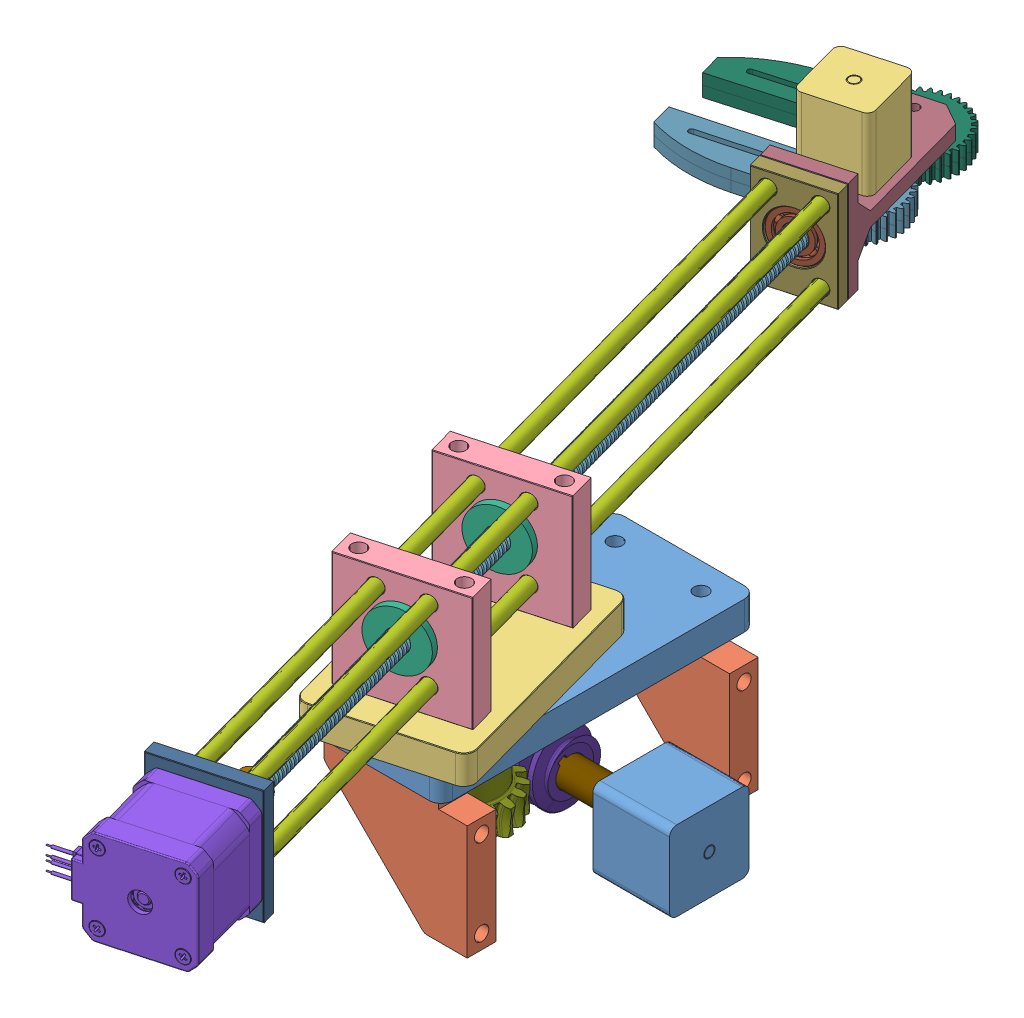
SolidWorks assembly CubeClawAssy, configuration Default. Lengths in mm.
Overall size (227.38 147.32 508.61).
29 component instances, 21 part files, 65 mates.
Components (placement in the parent):
- ClawArmBearingMount-1: ClawArmBearingMount [Default] at (-152.4 31.877 44.45) x (0 0 1) z (-1 0 0) size (139.7 12.7 63.5)
- 60355K509_BALL BEARING-1: 60355K509_BALL BEARING [60355K509] at (-152.4 36.6395 73.406) x (-0.297226 0 -0.954807) z (0 1 0) size (50.8 50.8 9.53)
- ArmRotate-1: ArmRotate [Default] at (-152.4 57.277 73.406) x (0.265648 0 0.96407) z (0.96407 0 -0.265648) size (101.6 63.5 63.5)
- RackStand-1: RackStand [Default] at (-160.8343 57.277 42.7968) x (0.265648 0 0.96407) z (-0.96407 0 0.265648) size (12 50.8 50.8)
- RackStand-2: RackStand [Default] at (-143.9657 57.277 104.0152) x (0.265648 0 0.96407) z (-0.96407 0 0.265648) size (12 50.8 50.8)
- 93410A912_ASTM A193 STEEL ACME LEAD SCREW-1: 93410A912_ASTM A193 STEEL ACME LEAD SCREW [93410A912] at (-159.5487 84.582 47.4626) x (0.957787 0.113984 -0.263917) z (-0.265648 0 -0.96407) size (11 9.53 384.84)
- 95120A592_BRONZE GENERAL PURPOSE ACME FLANGE NUT-1: 95120A592_BRONZE GENERAL PURPOSE ACME FLANGE NUT [95120A592] at (-158.3968 84.582 51.643) x (0.935858 -0.240148 -0.257875) z (0.231519 0.970736 -0.063795) size (25.4 22.84 25.4)
- 95120A592_BRONZE GENERAL PURPOSE ACME FLANGE NUT-2: 95120A592_BRONZE GENERAL PURPOSE ACME FLANGE NUT [95120A592] at (-141.5281 84.582 112.8615) x (0.890426 -0.383331 -0.245356) z (0.369558 0.923611 -0.101831) size (25.4 22.84 25.4)
- Rail-1: Rail [Default] at (-200.9719 68.707 -138.723) x (0.963827 0.022472 -0.265581) z (0.265648 0 0.96407) size (6.35 6.35 381)
- Rail-2: Rail [Default] at (-219.3375 68.707 -133.6624) x (0.963827 0.022472 -0.265581) z (0.265648 0 0.96407) size (6.35 6.35 381)
- Rail-3: Rail [Default] at (-219.3375 100.457 -133.6624) x (-0.624115 0.762171 0.171974) z (0.265648 0 0.96407) size (6.35 6.35 381)
- Rail-4: Rail [Default] at (-200.9719 100.457 -138.723) x (0.963827 0.022472 -0.265581) z (0.265648 0 0.96407) size (6.35 6.35 381)
- nema_17_motor-1: nema_17_motor [Varsayılan] at (-108.9426 84.582 231.1179) x (0 -1 0) z (-0.265648 0 -0.96407) size (42 58.5 65.65)
- ClawWormCoupler-1: ClawWormCoupler [Default] at (-117.5497 84.582 199.8821) x (0.587821 0.792611 -0.161973) z (0.265648 0 0.96407) size (13.97 13.97 25.4)
- ClawRailMotorBracket-1: ClawRailMotorBracket [Default] at (-110.6295 84.582 224.9961) x (0.96407 0 -0.265648) z (0.265648 0 0.96407) size (43.18 50.8 6.35)
- 60355K504_BALL BEARING-1: 60355K504_BALL BEARING [60355K504] at (-209.4167 84.582 -133.5144) x (-0.963827 -0.022472 0.265581) z (0.265648 0 0.96407) size (22.23 22.23 5.56)
- ClawBracket-1: ClawBracket [Default] at (-210.1547 84.582 -136.1927) x (0.96407 0 -0.265648) z (0.265648 0 0.96407) size (31.75 44.45 6.35)
- ClawMount-1: ClawMount [Default] at (-194.8501 62.357 -140.4099) x (-0.96407 0 0.265648) z (-0.265648 0 -0.96407) size (31.75 44.45 76.2)
- CLAW_L-1: CLAW_L [Default] at (-218.589 76.6445 -166.8019) x (-0.262286 0 -0.96499) z (0 -1 0) size (40.21 91.53 4.76)
- CLAW_L-2: CLAW_L [Default] at (-218.589 81.407 -166.8019) x (-0.262286 0 -0.96499) z (0 -1 0) size (40.21 91.53 4.76)
- CLAW_R-1: CLAW_R [Default] at (-228.7102 76.6445 -203.533) x (-0.274481 0 -0.961592) z (0 -1 0) size (40.15 91.5 4.76)
- CLAW_R-2: CLAW_R [Default] at (-228.7102 81.407 -203.533) x (-0.274481 0 -0.961592) z (0 -1 0) size (40.15 91.5 4.76)
- 57545K511_SPEED-REDUCING WORM GEAR FOR 90 DEG TRANSFER-1: 57545K511_SPEED-REDUCING WORM GEAR FOR 90 DEG TRANSFER [57545K511] at (-152.4 0.127 73.406) x (-0.122179 0 0.992508) z (-0.992508 0 -0.122179) size (44.78 28.61 44.18)
- 57545K527_SPEED-REDUCING WORM GEAR FOR 90 DEG TRANSFER-2: 57545K527_SPEED-REDUCING WORM GEAR FOR 90 DEG TRANSFER [57545K527] at (-151.281 0.382 40.4015) x (0 0.509771 -0.86031) z (1 0 0) size (31.13 29.72 30.93)
- RotationBushing-1: RotationBushing [Default] at (-111.5935 0.382 40.4015) x (0 -0.164114 0.986441) z (-1 0 0) size (12.7 12.7 53.98)
- 6627T380_POSITION-CONTROL DC MOTOR-1: 6627T380_POSITION-CONTROL DC MOTOR [6627T38] at (-109.5615 0.382 40.4015) x (0 0 1) z (-1 0 0) size (35.31 35.31 49.28)
- CubeArmMountBracket-3: CubeArmMountBracket [Default] at (-127 25.527 -7.3307) x (0 -1 0) z (0 0 -1) size (57.15 63.5 12.7)
- CubeArmMountBracket-4: CubeArmMountBracket [Default] at (-127 25.273 109.0013) x (0 -1 0) z (0 0 -1) size (57.15 63.5 12.7)
- 6627T370_POSITION-CONTROL DC MOTOR-1: 6627T370_POSITION-CONTROL DC MOTOR [6627T37] at (-218.589 89.789 -166.8019) x (0.96407 0 -0.265648) z (0 -1 0) size (28.19 28.19 52.07)
Mates (geometry in assembly coordinates):
- Coincident4: coincident aligned: plane of ClawArmBearingMount-1 through (-152.4 31.877 44.45) normal (0 -1 0); plane of 60355K509_BALL BEARING-1 through (-176.1974 31.877 80.814) normal (0 -1 0)
- Concentric8: concentric aligned: cylinder of 60355K509_BALL BEARING-1 through (-152.4 41.402 73.406) axis (0 1 0) radius 12.7; cylinder of ArmRotate-1 through (-152.4 -6.223 73.406) axis (0 1 0) radius 12.7
- Coincident5: coincident anti-aligned: plane of ClawArmBearingMount-1 through (-152.4 44.577 44.45) normal (0 1 0); plane of ArmRotate-1 through (-152.4 44.577 73.406) normal (0 -1 0)
- Concentric9: concentric anti-aligned: cylinder of ArmRotate-1 through (-142.4688 44.577 37.7362) axis (0 1 0) radius 3.175; cylinder of RackStand-1 through (-142.4688 108.077 37.7362) axis (0 -1 0) radius 3.175
- Coincident6: coincident anti-aligned: plane of ArmRotate-1 through (-152.4 57.277 73.406) normal (0 1 0); plane of RackStand-1 through (-160.8343 57.277 42.7968) normal (0 -1 0)
- Concentric10: concentric anti-aligned: cylinder of ArmRotate-1 through (-179.1999 44.577 47.8574) axis (0 1 0) radius 3.175; cylinder of RackStand-1 through (-179.1999 108.077 47.8574) axis (0 -1 0) radius 3.175
- Concentric11: concentric anti-aligned: cylinder of ArmRotate-1 through (-162.3312 44.577 109.0758) axis (0 1 0) radius 3.3492; cylinder of RackStand-2 through (-162.3312 108.077 109.0758) axis (0 -1 0) radius 3.175
- Coincident7: coincident anti-aligned: plane of ArmRotate-1 through (-152.4 57.277 73.406) normal (0 1 0); plane of RackStand-2 through (-143.9657 57.277 104.0152) normal (0 -1 0)
- Concentric12: concentric anti-aligned: cylinder of ArmRotate-1 through (-125.6001 44.577 98.9546) axis (0 1 0) radius 3.175; cylinder of RackStand-2 through (-125.6001 108.077 98.9546) axis (0 -1 0) radius 3.175
- Concentric13: concentric anti-aligned: circle of RackStand-1; circle of 93410A912_ASTM A193 STEEL ACME LEAD SCREW-1
- Concentric14: concentric anti-aligned: cylinder of RackStand-1 through (-172.7351 84.582 -0.3926) axis (0.265648 0 0.96407) radius 6.35; cylinder of 95120A592_BRONZE GENERAL PURPOSE ACME FLANGE NUT-1 through (-148.759 84.582 86.6197) axis (-0.265648 0 -0.96407) radius 6.35
- Coincident9: coincident anti-aligned: plane of RackStand-1 through (-183.7276 108.077 55.3296) normal (0.265648 0 0.96407); plane of 95120A592_BRONZE GENERAL PURPOSE ACME FLANGE NUT-1 through (-159.2402 84.582 48.5821) normal (-0.265648 0 -0.96407)
- Concentric16: concentric anti-aligned: cylinder of RackStand-2 through (-155.8665 84.582 60.8258) axis (0.265648 0 0.96407) radius 6.35; cylinder of 95120A592_BRONZE GENERAL PURPOSE ACME FLANGE NUT-2 through (-131.8903 84.582 147.8382) axis (-0.265648 0 -0.96407) radius 6.35
- Coincident10: coincident anti-aligned: plane of RackStand-2 through (-166.8589 108.077 116.548) normal (0.265648 0 0.96407); plane of 95120A592_BRONZE GENERAL PURPOSE ACME FLANGE NUT-2 through (-142.3715 84.582 109.8006) normal (-0.265648 0 -0.96407)
- Concentric17: concentric anti-aligned: cylinder of RackStand-1 through (-181.9179 100.457 2.1377) axis (0.265648 0 0.96407) radius 3.175; cylinder of Rail-3 through (-118.1254 100.457 233.6482) axis (-0.265648 0 -0.96407) radius 3.175
- Concentric18: concentric anti-aligned: cylinder of RackStand-1 through (-163.5524 100.457 -2.9229) axis (0.265648 0 0.96407) radius 3.175; cylinder of Rail-4 through (-99.7599 100.457 228.5876) axis (-0.265648 0 -0.96407) radius 3.175
- Concentric19: concentric anti-aligned: cylinder of RackStand-1 through (-181.9179 68.707 2.1377) axis (0.265648 0 0.96407) radius 3.175; cylinder of Rail-2 through (-118.1254 68.707 233.6482) axis (-0.265648 0 -0.96407) radius 3.175
- Concentric20: concentric anti-aligned: cylinder of RackStand-1 through (-163.5524 68.707 -2.9229) axis (0.265648 0 0.96407) radius 3.175; cylinder of Rail-1 through (-99.7599 68.707 228.5876) axis (-0.265648 0 -0.96407) radius 3.175
- Coincident11: coincident aligned: plane of Rail-1 through (-99.7599 68.707 228.5876) normal (0.265648 0 0.96407); plane of Rail-2 through (-118.1254 68.707 233.6482) normal (0.265648 0 0.96407)
- Coincident12: coincident aligned: plane of Rail-2 through (-118.1254 68.707 233.6482) normal (0.265648 0 0.96407); plane of Rail-3 through (-118.1254 100.457 233.6482) normal (0.265648 0 0.96407)
- Coincident13: coincident aligned: plane of Rail-3 through (-118.1254 100.457 233.6482) normal (0.265648 0 0.96407); plane of Rail-4 through (-99.7599 100.457 228.5876) normal (0.265648 0 0.96407)
- Coincident14: coincident aligned: plane of 93410A912_ASTM A193 STEEL ACME LEAD SCREW-1 through (-108.9426 84.582 231.1179) normal (0.265648 0 0.96407); plane of Rail-2 through (-118.1254 68.707 233.6482) normal (0.265648 0 0.96407)
- Concentric21: concentric anti-aligned: circle of 93410A912_ASTM A193 STEEL ACME LEAD SCREW-1; cylinder of ClawWormCoupler-1 through (-110.8022 84.582 224.3694) axis (-0.265648 0 -0.96407) radius 2.54
- Concentric22: concentric anti-aligned: cylinder of nema_17_motor-1 through (-115.5839 84.582 207.0162) axis (0.265648 0 0.96407) radius 2.5; cylinder of ClawWormCoupler-1 through (-110.8022 84.582 224.3694) axis (-0.265648 0 -0.96407) radius 2.54
- Coincident15: coincident anti-aligned: plane of nema_17_motor-1 through (-110.8022 84.582 224.3694) normal (-0.265648 0 -0.96407); plane of ClawWormCoupler-1 through (-110.8022 84.582 224.3694) normal (0.265648 0 0.96407)
- Coincident16: coincident aligned: plane of Rail-2 through (-118.1254 68.707 233.6482) normal (0.265648 0 0.96407); plane of ClawRailMotorBracket-1 through (-108.9426 84.582 231.1179) normal (0.265648 0 0.96407)
- Concentric26: concentric aligned: cylinder of Rail-2 through (-118.1254 68.707 233.6482) axis (-0.265648 0 -0.96407) radius 3.175; cylinder of ClawRailMotorBracket-1 through (-118.1254 68.707 233.6482) axis (-0.265648 0 -0.96407) radius 3.175
- Concentric27: concentric aligned: cylinder of Rail-4 through (-99.7599 100.457 228.5876) axis (-0.265648 0 -0.96407) radius 3.175; cylinder of ClawRailMotorBracket-1 through (-99.7599 100.457 228.5876) axis (-0.265648 0 -0.96407) radius 3.175
- Parallel4: parallel aligned: cylinder of nema_17_motor-1 through (-123.8857 69.082 235.2355) axis (-0.265648 0 -0.96407) radius 1.25; cylinder of ClawRailMotorBracket-1 through (-123.8799 100.076 235.2339) axis (-0.265648 0 -0.96407) radius 1.524
- Coincident17: coincident anti-aligned: plane of nema_17_motor-1 through (-108.9426 84.582 231.1179) normal (-0.265648 0 -0.96407); plane of ClawRailMotorBracket-1 through (-108.9426 84.582 231.1179) normal (0.265648 0 0.96407)
- Parallel5: parallel aligned: line of nema_17_motor-1 through (-129.1084 100.9536 236.9858) axis (0 -1 0); line of ClawRailMotorBracket-1 through (-131.3763 109.982 230.9763) axis (0 -1 0)
- Coincident19: coincident aligned: plane of Rail-1 through (-200.9719 68.707 -138.723) normal (-0.265648 0 -0.96407); plane of 60355K504_BALL BEARING-1 through (-210.0455 79.543 -136.2228) normal (-0.265648 0 -0.96407)
- Coincident20: coincident anti-aligned: plane of 93410A912_ASTM A193 STEEL ACME LEAD SCREW-1 through (-210.1547 84.582 -136.1927) normal (-0.265648 0 -0.96407); circle of 60355K504_BALL BEARING-1
- Concentric29: concentric aligned: cylinder of Rail-3 through (-118.1254 100.457 233.6482) axis (-0.265648 0 -0.96407) radius 3.175; cylinder of ClawBracket-1 through (-217.6506 100.457 -127.5406) axis (-0.265648 0 -0.96407) radius 3.175
- Concentric30: concentric aligned: cylinder of Rail-4 through (-99.7599 100.457 228.5876) axis (-0.265648 0 -0.96407) radius 3.175; cylinder of ClawBracket-1 through (-199.2851 100.457 -132.6012) axis (-0.265648 0 -0.96407) radius 3.175
- Coincident21: coincident aligned: plane of Rail-3 through (-219.3375 100.457 -133.6624) normal (-0.265648 0 -0.96407); plane of ClawBracket-1 through (-210.1547 84.582 -136.1927) normal (-0.265648 0 -0.96407)
- Concentric31: concentric aligned: cylinder of Rail-3 through (-118.1254 100.457 233.6482) axis (-0.265648 0 -0.96407) radius 3.175; cylinder of ClawMount-1 through (-215.9637 100.457 -121.4187) axis (-0.265648 0 -0.96407) radius 3.175
- Concentric32: concentric aligned: cylinder of Rail-4 through (-99.7599 100.457 228.5876) axis (-0.265648 0 -0.96407) radius 3.175; cylinder of ClawMount-1 through (-197.5982 100.457 -126.4793) axis (-0.265648 0 -0.96407) radius 3.175
- Coincident22: coincident anti-aligned: plane of ClawBracket-1 through (-210.1547 84.582 -136.1927) normal (-0.265648 0 -0.96407); plane of ClawMount-1 through (-225.4593 62.357 -131.9756) normal (0.265648 0 0.96407)
- Coincident23: coincident anti-aligned: plane of ClawMount-1 through (-245.7017 81.407 -205.4377) normal (0 -1 0); plane of CLAW_L-2 through (-218.589 81.407 -166.8019) normal (0 1 0)
- Concentric33: concentric anti-aligned: circle of ClawMount-1; circle of CLAW_L-2
- Coincident24: coincident anti-aligned: plane of CLAW_L-1 through (-218.589 76.6445 -166.8019) normal (0 1 0); plane of CLAW_L-2 through (-218.589 76.6445 -166.8019) normal (0 -1 0)
- Concentric34: concentric aligned: circle of CLAW_L-1; circle of CLAW_L-2
- Parallel6: parallel aligned: line of CLAW_L-1 through (-236.2483 71.882 -170.2144) axis (-0.96499 0 0.262286); line of CLAW_L-2 through (-236.2483 76.6445 -170.2144) axis (-0.96499 0 0.262286)
- Coincident27: coincident anti-aligned: plane of ClawMount-1 through (-245.7017 81.407 -205.4377) normal (0 -1 0); plane of CLAW_R-2 through (-228.7102 81.407 -203.533) normal (0 1 0)
- Concentric35: concentric anti-aligned: circle of ClawMount-1; circle of CLAW_R-2
- Coincident28: coincident anti-aligned: plane of CLAW_R-1 through (-228.7102 76.6445 -203.533) normal (0 1 0); plane of CLAW_R-2 through (-228.7102 76.6445 -203.533) normal (0 -1 0)
- Concentric36: concentric aligned: circle of CLAW_R-1; circle of CLAW_R-2
- Coincident31: coincident aligned: line of CLAW_R-1 through (-244.3017 76.6445 -190.8412) axis (-0.961592 0 0.274481); line of CLAW_R-2 through (-244.3017 76.6445 -190.8412) axis (-0.961592 0 0.274481)
- Concentric38: concentric anti-aligned: cylinder of 60355K504_BALL BEARING-1 through (-208.6787 84.582 -130.8361) axis (0.265648 0 0.96407) radius 11.1125; cylinder of ClawBracket-1 through (-208.4678 84.582 -130.0709) axis (-0.265648 0 -0.96407) radius 11.176
- Concentric39: concentric aligned: cylinder of ArmRotate-1 through (-152.4 22.352 73.406) axis (0 -1 0) radius 6.35; cylinder of 57545K511_SPEED-REDUCING WORM GEAR FOR 90 DEG TRANSFER-1 through (-152.4 -67.3016 73.406) axis (0 -1 0) radius 6.35
- Coincident33: coincident anti-aligned: plane of ArmRotate-1 through (-152.4 22.352 73.406) normal (0 -1 0); plane of 57545K511_SPEED-REDUCING WORM GEAR FOR 90 DEG TRANSFER-1 through (-152.4 22.352 73.406) normal (0 1 0)
- Concentric43: concentric aligned: cylinder of 57545K527_SPEED-REDUCING WORM GEAR FOR 90 DEG TRANSFER-2 through (-151.281 0.382 40.4015) axis (1 0 0) radius 6.35; cylinder of RotationBushing-1 through (-165.5685 0.382 40.4015) axis (1 0 0) radius 6.35
- Concentric49: concentric anti-aligned: cylinder of RotationBushing-1 through (-165.5685 0.382 40.4015) axis (1 0 0) radius 2.54; cylinder of 6627T380_POSITION-CONTROL DC MOTOR-1 through (-124.8015 0.382 40.4015) axis (-1 0 0) radius 2.4994
- Concentric56: concentric anti-aligned: cylinder of ClawArmBearingMount-1 through (-152.4 44.577 73.406) axis (0 -1 0) radius 25.654; cylinder of 60355K509_BALL BEARING-1 through (-152.4 41.402 73.406) axis (0 1 0) radius 25.4
- Concentric66: concentric anti-aligned: cylinder of ClawArmBearingMount-1 through (-171.45 44.577 -13.716) axis (0 -1 0) radius 3.175; cylinder of CubeArmMountBracket-3 through (-171.45 17.907 -13.716) axis (0 1 0) radius 3.175
- Concentric67: concentric anti-aligned: cylinder of ClawArmBearingMount-1 through (-133.35 44.577 -13.716) axis (0 -1 0) radius 3.175; cylinder of CubeArmMountBracket-3 through (-133.35 17.907 -13.716) axis (0 1 0) radius 3.175
- Concentric68: concentric anti-aligned: cylinder of ClawArmBearingMount-1 through (-133.35 44.577 -13.716) axis (0 -1 0) radius 3.175; cylinder of CubeArmMountBracket-3 through (-133.35 17.907 -13.716) axis (0 1 0) radius 3.175
- Concentric69: concentric anti-aligned: cylinder of ClawArmBearingMount-1 through (-171.45 44.577 -13.716) axis (0 -1 0) radius 3.175; cylinder of CubeArmMountBracket-3 through (-171.45 17.907 -13.716) axis (0 1 0) radius 3.175
- Coincident57: coincident anti-aligned: plane of ClawArmBearingMount-1 through (-152.4 31.877 44.45) normal (0 -1 0); plane of CubeArmMountBracket-3 through (-127 31.877 -7.3307) normal (0 1 0)
- Coincident58: coincident anti-aligned: plane of RotationBushing-1 through (-111.5935 0.382 40.4015) normal (1 0 0); plane of 6627T380_POSITION-CONTROL DC MOTOR-1 through (-111.5935 0.382 40.4015) normal (-1 0 0)
- Coincident59: coincident aligned: plane of 57545K527_SPEED-REDUCING WORM GEAR FOR 90 DEG TRANSFER-2 through (-165.5685 0.382 40.4015) normal (-1 0 0); plane of RotationBushing-1 through (-165.5685 0.382 40.4015) normal (-1 0 0)
- Concentric71: concentric anti-aligned: cylinder of ClawMount-1 through (-218.589 68.707 -166.8019) axis (0 1 0) radius 2.1828; cylinder of 6627T370_POSITION-CONTROL DC MOTOR-1 through (-218.589 69.723 -166.8019) axis (0 -1 0) radius 2.4994
- Parallel8: parallel anti-aligned: line of ClawMount-1 through (-198.6287 87.757 -154.1228) axis (-0.265648 0 -0.96407); line of 6627T370_POSITION-CONTROL DC MOTOR-1 through (-207.9 89.789 -181.0764) axis (0.265648 0 0.96407)
- Coincident63: coincident aligned: plane of ClawMount-1 through (-227.1462 87.757 -138.0974) normal (0 1 0); circle of 6627T370_POSITION-CONTROL DC MOTOR-1
